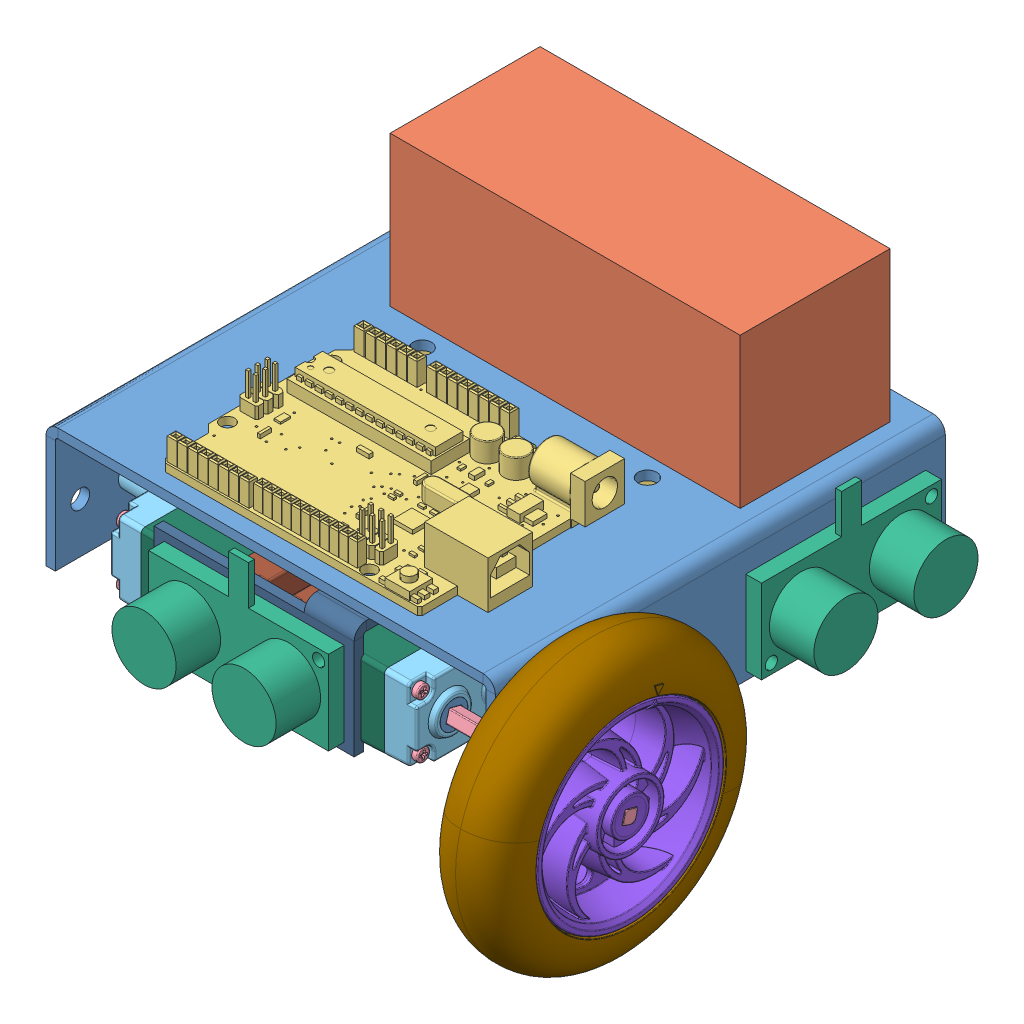
SolidWorks assembly mte380_Assy_02_minibot_01, configuration Default. Lengths in mm.
Overall size (142.74 102.26 150.9).
73 component instances, 28 part files, 30 mates.
Components (placement in the parent):
- mte380_02_frame_02-1: mte380_02_frame_02 [Default] at (-29.7082 71.1875 142.7924) size (114.15 31.84 114.3)
- mte380_02_package_01-1: mte380_02_package_01 [Default] at (19.4156 73.194 94.9023) size (88.9 38.1 38.1)
- Arduino-1: Arduino [Predeterminado] at (59.6024 71.1875 132.4413) x (-0.999979 0 0.006548) z (-0.006548 0 -0.999979) size (75 12 51.02)
- mte380_01_vex_motor_269-1: mte380_01_vex_motor_269 [Default] at (45.1052 52.051 144.3626) x (0 0 1) z (1 0 0) size (46.4 20.59 51.81)
  - SPPM206-0150BO-1: SPPM206-0150BO [Default] at (17.3 7.3 -1.5) x (1 0 0) z (0 -1 0) size (3.3 16.36 3.3)
  - 276-2181-003 Rev1-1: 276-2181-003 Rev1 [Default] at (0 0 -28) size (38.95 18.95 25.5)
  - 276-2177-019 Rev1-1: 276-2177-019 Rev1 [Default] at (-14.2702 0 -28) x (0.144195 -0.989549 0) z (0.989549 0.144195 0) size (6.3 15.8 6.3)
  - 276-2181-011 Rev1-1: 276-2181-011 Rev1 [Default] at (11.1298 0 -11) x (-1 0 0) z (0 1 0) size (11 4 11)
  - QFK-N30QAV-16068-1: QFK-N30QAV-16068 [Default] at (-12.9 0 -23) x (0 1 0) z (0 0 1) size (12 10 26.1)
  - SPPM143-0030BO-1: SPPM143-0030BO [Default] at (-12.9 4.25 -6) x (-1 0 0) z (0 1 0) size (2.4 6.08 2.4)
  - 276-2181-010 Rev1-1: 276-2181-010 Rev1 [Default] at (10.8763 0 -9.4) x (0.878827 0.47714 0) z (0 0 1) size (1.5 1.5 16)
  - 276-2181-001 Rev1-1: 276-2181-001 Rev1 [Default] at origin size (40 20 8.01)
  - 276-2181-006 Rev1-1: 276-2181-006 Rev1 [Default] at (10.8763 0 -1.05) x (-0.259931 -0.965627 0) z (0 0 1) size (14.22 14.25 6.9)
  - 276-2181-007 Rev1-1: 276-2181-007 Rev1 [Default] at (2.1533 -1.4937 -4.4) x (-0.202497 0.979283 0) z (0 0 1) size (14.22 14.25 14.9)
  - 276-2181-010 Rev1-2: 276-2181-010 Rev1 [Default] at (-5.7003 2.586 -9.4) size (1.5 1.5 16)
  - 276-2177-018 Rev1-1: 276-2177-018 Rev1 [Default] at (-18.5 0.1 2.5) x (0 1 0) z (1 0 0) size (6.82 4.47 8.9)
  - 276-2181-006 Rev1-2: 276-2181-006 Rev1 [Default] at (2.1533 -1.4937 2.75) x (-0.071378 0.997449 0) z (0 0 1) size (14.22 14.25 6.9)
  - 276-2181-002 Rev1-1: 276-2181-002 Rev1 [Default] at (0 0 -20) size (40 20 23)
  - 276-2181-009 Rev1-1: 276-2181-009 Rev1 [Default] at (2.1533 -1.4937 -26.5) size (1.5 1.5 33)
  - SPPM206-0150BO-2: SPPM206-0150BO [Default] at (-16.9263 6.9263 -18.5) x (-0.075705 0.99713 0) z (-0.99713 -0.075705 0) size (3.3 16.36 3.3)
  - 276-2181-011 Rev1-2: 276-2181-011 Rev1 [Default] at (11.1298 0 -24) x (-0.997622 -0.068917 0) z (-0.068917 0.997622 0) size (11 4 11)
  - 276-2177-019 Rev1-2: 276-2177-019 Rev1 [Default] at (-1.5702 0 -28) x (0.32391 -0.946088 0) z (0.946088 0.32391 0) size (6.3 15.8 6.3)
  - SPPM206-0150BO-3: SPPM206-0150BO [Default] at (-17.3 -7.3 -1.5) x (0.292947 -0.956129 0) z (-0.956129 -0.292947 0) size (3.3 16.36 3.3)
  - SPPM206-0150BO-4: SPPM206-0150BO [Default] at (16.9263 -6.9263 -18.5) x (0.149257 -0.988799 0) z (0.988799 0.149257 0) size (3.3 16.36 3.3)
  - SPPM206-0150BO-5: SPPM206-0150BO [Default] at (17.3 -7.3 -1.5) x (1 0 0) z (0 -1 0) size (3.3 16.36 3.3)
  - SPPM206-0150BO-6: SPPM206-0150BO [Default] at (-16.9263 -6.9263 -18.5) x (-0.049887 0.998755 0) z (-0.998755 -0.049887 0) size (3.3 16.36 3.3)
  - SPPM206-0150BO-7: SPPM206-0150BO [Default] at (-17.3 7.3 -1.5) x (-0.963198 0.268794 0) z (0.268794 0.963198 0) size (3.3 16.36 3.3)
  - SPPM206-0150BO-8: SPPM206-0150BO [Default] at (16.9263 6.9263 -18.5) x (0.906825 0.421508 0) z (-0.421508 0.906825 0) size (3.3 16.36 3.3)
  - SPPM143-0030BO-2: SPPM143-0030BO [Default] at (-12.9 -4.25 -6) x (-0.988208 -0.153116 0) z (-0.153116 0.988208 0) size (2.4 6.08 2.4)
  - 276-2181-004 Rev1-1: 276-2181-004 Rev1 [Default] at (-12.9 0 -0.1) x (0.94341 -0.331628 0) z (0 0 -1) size (5.17 5.4 3)
  - 276-2181-005 Rev1-1: 276-2181-005 Rev1 [Default] at (-5.7003 2.586 -0.05) x (0.460478 -0.887671 0) z (0 0 1) size (11.88 11.88 5.9)
  - 276-2181-008 Rev1_276-2181-008g-1: 276-2181-008 Rev1_276-2181-008g [Default] at (11.1298 0 -14.5) x (0.267616 -0.963526 0) z (0 0 -1) size (13.83 13.88 17.3)
  - 276-2181-012 Rev1-1: 276-2181-012 Rev1 [Default] at (-12.9 0 -24) size (13.6 13 1)
- mte380_01_vex_motor_269-2: mte380_01_vex_motor_269 [Default] at (66.9284 52.051 144.3626) x (0 0 1) z (-1 0 0) size (46.4 20.59 51.81)
  - SPPM206-0150BO-1: SPPM206-0150BO [Default] at (17.3 7.3 -1.5) x (1 0 0) z (0 -1 0) size (3.3 16.36 3.3)
  - 276-2181-003 Rev1-1: 276-2181-003 Rev1 [Default] at (0 0 -28) size (38.95 18.95 25.5)
  - 276-2177-019 Rev1-1: 276-2177-019 Rev1 [Default] at (-14.2702 0 -28) x (0.144195 -0.989549 0) z (0.989549 0.144195 0) size (6.3 15.8 6.3)
  - 276-2181-011 Rev1-1: 276-2181-011 Rev1 [Default] at (11.1298 0 -11) x (-1 0 0) z (0 1 0) size (11 4 11)
  - QFK-N30QAV-16068-1: QFK-N30QAV-16068 [Default] at (-12.9 0 -23) x (0 1 0) z (0 0 1) size (12 10 26.1)
  - SPPM143-0030BO-1: SPPM143-0030BO [Default] at (-12.9 4.25 -6) x (-1 0 0) z (0 1 0) size (2.4 6.08 2.4)
  - 276-2181-010 Rev1-1: 276-2181-010 Rev1 [Default] at (10.8763 0 -9.4) x (0.878827 0.47714 0) z (0 0 1) size (1.5 1.5 16)
  - 276-2181-001 Rev1-1: 276-2181-001 Rev1 [Default] at origin size (40 20 8.01)
  - 276-2181-006 Rev1-1: 276-2181-006 Rev1 [Default] at (10.8763 0 -1.05) x (-0.259931 -0.965627 0) z (0 0 1) size (14.22 14.25 6.9)
  - 276-2181-007 Rev1-1: 276-2181-007 Rev1 [Default] at (2.1533 -1.4937 -4.4) x (-0.202497 0.979283 0) z (0 0 1) size (14.22 14.25 14.9)
  - 276-2181-010 Rev1-2: 276-2181-010 Rev1 [Default] at (-5.7003 2.586 -9.4) size (1.5 1.5 16)
  - 276-2177-018 Rev1-1: 276-2177-018 Rev1 [Default] at (-18.5 0.1 2.5) x (0 1 0) z (1 0 0) size (6.82 4.47 8.9)
  - 276-2181-006 Rev1-2: 276-2181-006 Rev1 [Default] at (2.1533 -1.4937 2.75) x (-0.071378 0.997449 0) z (0 0 1) size (14.22 14.25 6.9)
  - 276-2181-002 Rev1-1: 276-2181-002 Rev1 [Default] at (0 0 -20) size (40 20 23)
  - 276-2181-009 Rev1-1: 276-2181-009 Rev1 [Default] at (2.1533 -1.4937 -26.5) size (1.5 1.5 33)
  - SPPM206-0150BO-2: SPPM206-0150BO [Default] at (-16.9263 6.9263 -18.5) x (-0.075705 0.99713 0) z (-0.99713 -0.075705 0) size (3.3 16.36 3.3)
  - 276-2181-011 Rev1-2: 276-2181-011 Rev1 [Default] at (11.1298 0 -24) x (-0.997622 -0.068917 0) z (-0.068917 0.997622 0) size (11 4 11)
  - 276-2177-019 Rev1-2: 276-2177-019 Rev1 [Default] at (-1.5702 0 -28) x (0.32391 -0.946088 0) z (0.946088 0.32391 0) size (6.3 15.8 6.3)
  - SPPM206-0150BO-3: SPPM206-0150BO [Default] at (-17.3 -7.3 -1.5) x (0.292947 -0.956129 0) z (-0.956129 -0.292947 0) size (3.3 16.36 3.3)
  - SPPM206-0150BO-4: SPPM206-0150BO [Default] at (16.9263 -6.9263 -18.5) x (0.149257 -0.988799 0) z (0.988799 0.149257 0) size (3.3 16.36 3.3)
  - SPPM206-0150BO-5: SPPM206-0150BO [Default] at (17.3 -7.3 -1.5) x (1 0 0) z (0 -1 0) size (3.3 16.36 3.3)
  - SPPM206-0150BO-6: SPPM206-0150BO [Default] at (-16.9263 -6.9263 -18.5) x (-0.049887 0.998755 0) z (-0.998755 -0.049887 0) size (3.3 16.36 3.3)
  - SPPM206-0150BO-7: SPPM206-0150BO [Default] at (-17.3 7.3 -1.5) x (-0.963198 0.268794 0) z (0.268794 0.963198 0) size (3.3 16.36 3.3)
  - SPPM206-0150BO-8: SPPM206-0150BO [Default] at (16.9263 6.9263 -18.5) x (0.906825 0.421508 0) z (-0.421508 0.906825 0) size (3.3 16.36 3.3)
  - SPPM143-0030BO-2: SPPM143-0030BO [Default] at (-12.9 -4.25 -6) x (-0.988208 -0.153116 0) z (-0.153116 0.988208 0) size (2.4 6.08 2.4)
  - 276-2181-004 Rev1-1: 276-2181-004 Rev1 [Default] at (-12.9 0 -0.1) x (0.94341 -0.331628 0) z (0 0 -1) size (5.17 5.4 3)
  - 276-2181-005 Rev1-1: 276-2181-005 Rev1 [Default] at (-5.7003 2.586 -0.05) x (0.460478 -0.887671 0) z (0 0 1) size (11.88 11.88 5.9)
  - 276-2181-008 Rev1_276-2181-008g-1: 276-2181-008 Rev1_276-2181-008g [Default] at (11.1298 0 -14.5) x (0.267616 -0.963526 0) z (0 0 -1) size (13.83 13.88 17.3)
  - 276-2181-012 Rev1-1: 276-2181-012 Rev1 [Default] at (-12.9 0 -24) size (13.6 13 1)
- mte380_01_reedy_battery_pack-1: mte380_01_reedy_battery_pack [Default] at (99.1968 68.8253 93.2624) x (-1 0 0) z (0 0 1) size (86.36 16.51 30.48)
- mte380_01_vex_shaft_2-1: mte380_01_vex_shaft_2 [Default] at (115.6284 52.0197 155.4747) x (0 -0.267616 -0.963526) z (1 0 0) size (4.18 4.18 51.01)
- mte380_01_vex_flat_bearing-2: mte380_01_vex_flat_bearing [Default] at (202.7526 39.351 169.2084) x (-1 0 0) z (0 -1 0) size (7.04 35.56 10.16)
- mte380_01_ultrasonic-1: mte380_01_ultrasonic [Default] at (113.0906 62.806 52.5424) x (0 0 1) z (0 1 0) size (45.7 15.3 31.3)
- mte380_vex_wheel-1: mte380_vex_wheel [Default] at (134.1635 32.8706 145.0423) x (0 -0.267616 -0.963526) z (1 0 0) size (69.86 69.86 20.66)
  - SMALL-WHEEL-RIM-1: SMALL-WHEEL-RIM [Default] at (-15.1515 15.6838 -2.6601) size (61.43 61.43 9.24)
  - SMALL-WHEEL-HUB-1: SMALL-WHEEL-HUB [Default] at (-15.1515 15.6838 -2.6601) size (61.36 61.43 20.66)
  - SMALL-WHEEL-TIRE-1: SMALL-WHEEL-TIRE [Default] at (-15.1515 15.6838 -2.6601) x (1 0 0) z (0 -1 0) size (69.86 19.99 69.86)
- mte380_02_front_ultrasonic_mount_01-1: mte380_02_front_ultrasonic_mount_01 [Default] at (30.312 40.3265 165.7389) x (1 0 0) z (0 -1 0) size (50.8 63.59 28.5)
- mte380_01_ultrasonic-2: mte380_01_ultrasonic [Default] at (78.592 63.6545 165.7389) x (-1 0 0) z (0 1 0) size (45.7 15.3 31.3)
Mates (geometry in assembly coordinates):
- Coincident6: coincident anti-aligned: plane of mte380_02_frame_02-1 through (-29.7082 68.8253 142.7924) normal (0 -1 0); plane of mte380_01_reedy_battery_pack-1 through (12.8368 68.8253 93.2624) normal (0 1 0)
- Concentric5: concentric aligned: circle of mte380_02_frame_02-1; circle of mte380_01_vex_flat_bearing-2
- Coincident11: coincident anti-aligned: plane of mte380_02_frame_02-1 through (113.0906 210.801 142.7924) normal (1 0 0); plane of mte380_01_vex_flat_bearing-2 through (113.0906 52.051 142.7924) normal (-1 0 0)
- Concentric6: concentric aligned: circle of mte380_02_frame_02-1; circle of mte380_01_vex_flat_bearing-2
- Coincident13: coincident anti-aligned: plane of mte380_01_vex_motor_269-2/276-2181-008 Rev1_276-2181-008g-1 through (90.2284 53.1734 153.5067) normal (0 0.267616 0.963526); plane of mte380_01_vex_shaft_2-1 through (141.0284 50.0653 154.37) normal (0 -0.267616 -0.963526)
- Coincident14: coincident anti-aligned: plane of mte380_01_vex_motor_269-2/276-2181-008 Rev1_276-2181-008g-1 through (90.2284 50.0653 154.37) normal (1 0 0); plane of mte380_01_vex_shaft_2-1 through (90.2284 53.9741 156.5795) normal (-1 0 0)
- Coincident15: coincident anti-aligned: plane of mte380_01_vex_motor_269-2/276-2181-008 Rev1_276-2181-008g-1 through (90.2284 50.9285 157.4781) normal (0 0.963526 -0.267616); plane of mte380_01_vex_shaft_2-1 through (141.0284 50.915 157.4292) normal (0 -0.963526 0.267616)
- Coincident16: coincident anti-aligned: plane of mte380_02_frame_02-1 through (113.0906 210.801 142.7924) normal (1 0 0); plane of mte380_01_ultrasonic-1 through (113.0906 62.806 52.5424) normal (-1 0 0)
- Concentric8: concentric aligned: circle of mte380_02_frame_02-1; circle of mte380_01_ultrasonic-1
- Concentric9: concentric anti-aligned: cylinder of mte380_02_frame_02-1 through (-1.057 44.006 95.7424) axis (1 0 0) radius 1.55; cylinder of mte380_01_ultrasonic-1 through (117.0906 44.006 95.7424) axis (-1 0 0) radius 1.55
- Coincident19: coincident anti-aligned: plane of mte380_01_vex_shaft_2-1 through (141.0284 50.915 157.4292) normal (0 0.267616 0.963526); plane of mte380_vex_wheel-1/SMALL-WHEEL-HUB-1 through (142.9334 54.0223 156.5661) normal (0 -0.267616 -0.963526)
- Coincident20: coincident anti-aligned: plane of mte380_01_vex_shaft_2-1 through (141.0284 50.915 157.4292) normal (0 -0.963526 0.267616); plane of mte380_vex_wheel-1/SMALL-WHEEL-HUB-1 through (142.9334 50.915 157.4292) normal (0 0.963526 -0.267616)
- Coincident21: coincident aligned: plane of mte380_vex_wheel-1/SMALL-WHEEL-HUB-1 through (141.0284 52.0371 155.4439) normal (1 0 0); plane of mte380_01_vex_shaft_2-1 through (141.0284 53.9741 156.5795) normal (1 0 0)
- Concentric10: concentric aligned: circle of mte380_02_frame_02-1; circle of Arduino-1
- Concentric11: concentric aligned: circle of mte380_02_frame_02-1; circle of Arduino-1
- Distance5: distance = 15.24 mm aligned: plane of mte380_01_reedy_battery_pack-1 through (12.8368 68.8253 62.7824) normal (0 0 -1); plane of mte380_02_frame_02-1 through (-29.7082 68.8253 47.5424) normal (0 0 -1)
- Width5: width aligned: plane of mte380_01_reedy_battery_pack-1 through (12.8368 68.8253 93.2624) normal (-1 0 0); plane of mte380_01_reedy_battery_pack-1 through (99.1968 68.8253 93.2624) normal (1 0 0); plane of mte380_02_frame_02-1 through (-1.057 39.351 142.7924) normal (-1 0 0); plane of mte380_02_frame_02-1 through (113.0906 210.801 142.7924) normal (1 0 0)
- Coincident28: coincident anti-aligned: plane of mte380_02_frame_02-1 through (-29.7082 71.1875 142.7924) normal (0 1 0); plane of Arduino-1 through (59.6024 71.1875 132.4413) normal (0 -1 0)
- Concentric13: concentric aligned: circle of mte380_02_frame_02-1; circle of mte380_02_front_ultrasonic_mount_01-1
- Concentric12: concentric aligned: circle of mte380_02_frame_02-1; circle of mte380_02_front_ultrasonic_mount_01-1
- Coincident31: coincident anti-aligned: plane of mte380_02_frame_02-1 through (-29.7082 68.8253 142.7924) normal (0 -1 0); plane of mte380_02_front_ultrasonic_mount_01-1 through (30.312 68.8253 191.0524) normal (0 1 0)
- Concentric14: concentric aligned: cylinder of mte380_02_front_ultrasonic_mount_01-1 through (35.392 44.8545 102.1514) axis (0 0 1) radius 1.55; circle of mte380_01_ultrasonic-2
- Concentric15: concentric aligned: circle of mte380_02_front_ultrasonic_mount_01-1; circle of mte380_01_ultrasonic-2
- Coincident34: coincident anti-aligned: plane of mte380_02_front_ultrasonic_mount_01-1 through (30.312 40.3265 165.7389) normal (0 0 1); plane of mte380_01_ultrasonic-2 through (78.592 63.6545 165.7389) normal (0 0 -1)
- Concentric16: concentric anti-aligned: circle of mte380_02_frame_02-1; circle of mte380_01_vex_motor_269-2/276-2181-003 Rev1-1
- Concentric17: concentric anti-aligned: circle of mte380_01_vex_flat_bearing-2; circle of mte380_01_vex_motor_269-2/276-2177-019 Rev1-1
- Coincident35: coincident anti-aligned: plane of mte380_02_frame_02-1 through (110.7284 210.801 142.7924) normal (-1 0 0); plane of mte380_01_vex_motor_269-2/276-2177-019 Rev1-1 through (110.7284 52.051 130.0924) normal (1 0 0)
- Concentric18: concentric: circle of mte380_02_frame_02-1; circle of mte380_01_vex_motor_269-1/276-2181-003 Rev1-1
- Coincident36: coincident: plane of mte380_02_frame_02-1 through (1.3052 39.351 142.7924) normal (1 0 0); plane of mte380_01_vex_motor_269-1/276-2177-019 Rev1-1 through (1.3052 33.2071 138.461) normal (-1 0 0)
- Concentric19: concentric anti-aligned: circle of mte380_02_frame_02-1; circle of mte380_01_vex_motor_269-1/276-2177-019 Rev1-1
